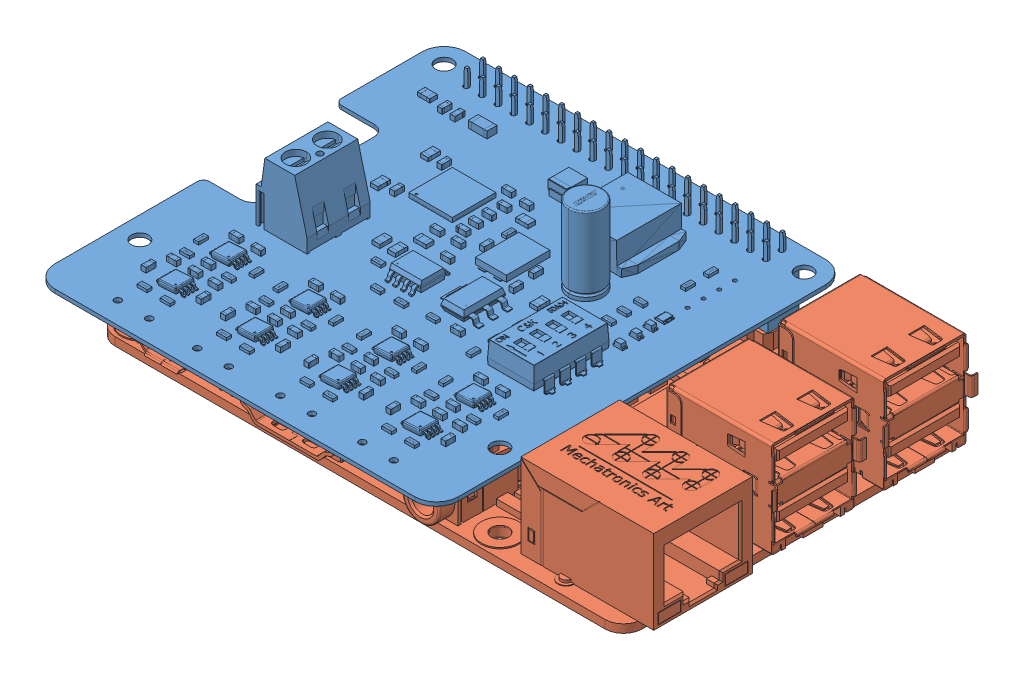
SolidWorks assembly pcbWithPi, configuration Default. Lengths in mm.
Overall size (89.64 41.22 66.33).
2 component instances, 2 part files, 3 mates.
Components (placement in the parent):
- Top-2: Top [Default] at (-0.258 29.0136 36.705) x (1 0 0) z (0 1 0) size (64.99 66.2 41.22)
- Raspberry Pi 3-2: Raspberry Pi 3 [Default] at (58.061 15.8899 -25.5913) x (1 0 0) z (0 1 0) size (89.64 57.31 18.59)
Mates (geometry in assembly coordinates):
- Coincident1: coincident anti-aligned: plane of Top-2 through (57.609 19.8899 -55.002) normal (0 0 1); plane of Raspberry Pi 3-2 through (31.4405 16.8799 -55.002) normal (0 0 -1)
- Coincident2: coincident anti-aligned: plane of Top-2 through (16.719 24.2132 -52.502) normal (1 0 0); plane of Raspberry Pi 3-2 through (16.719 16.8799 -53.868) normal (-1 0 0)
- Distance1: distance = 0.5 mm aligned: plane of Raspberry Pi 3-2 through (16.709 19.3899 -49.992) normal (0 1 0); plane of Top-2 through (57.609 19.8899 -50.002) normal (0 1 0)
